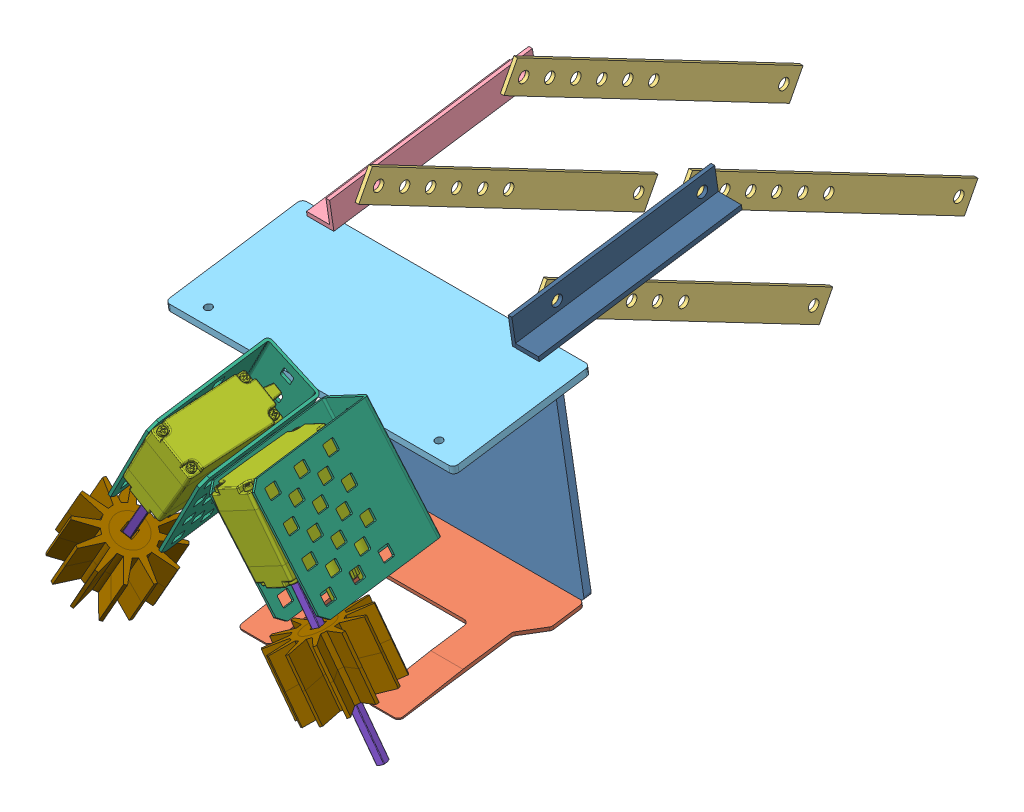
SolidWorks assembly Pyramid Intake, configuration Default. Lengths in mm.
Overall size (150.3 140.72 320.47).
19 component instances, 10 part files, 29 mates.
Components (placement in the parent):
- back-1: back [Default] at (51.2746 60.4405 44.4758) x (1 0 0) z (0 -0.146963 0.989142) size (85.5 99.5 3.17)
- BottomForklift-1: BottomForklift [Default] at (51.2746 -40.016 32.7601) x (1 0 0) z (0 -0.146963 0.989142) size (85.5 1.59 73.7)
- Circles 5.5in Inch Shaft Bar-1: Circles 5.5in Inch Shaft Bar [Default] at (81.5651 21.6246 -45.8337) x (0 0.885997 -0.463691) z (0 -0.463691 -0.885997) size (12.7 1.59 139.7)
- Circles 5.5in Inch Shaft Bar-2: Circles 5.5in Inch Shaft Bar [Default] at (81.5651 30.9788 -108.7925) x (0 0.885997 -0.463691) z (0 -0.463691 -0.885997) size (12.7 1.59 139.7)
- Circles 5.5in Inch Shaft Bar-3: Circles 5.5in Inch Shaft Bar [Default] at (1.9185 22.2168 -49.6344) x (0 0.885997 -0.463691) z (0 -0.463691 -0.885997) size (12.7 1.59 139.7)
- Circles 5.5in Inch Shaft Bar-4: Circles 5.5in Inch Shaft Bar [Default] at (1.9185 31.571 -112.5933) x (0 0.885997 -0.463691) z (0 -0.463691 -0.885997) size (12.7 1.59 139.7)
- Circles 3.5 inch Linkage-4: Circles 3.5 inch Linkage [Default] at (1.9185 61.0879 62.0444) x (0 0.989142 0.146963) z (0 -0.146963 0.989142) size (12.75 11.59 88.91)
- top-2: top [Default] at (45.9604 60.4405 44.4758) x (1 0 0) z (0 -0.146963 0.989142) size (125 3.17 60)
- VL-RACK-BRK RevA-1: VL-RACK-BRK RevA [Default] at (75.6784 37.9578 101.794) x (-0.866025 -0.494571 -0.073482) z (-0.5 0.856622 0.127274) size (24.56 52.4 50.8)
- VL-RACK-BRK RevA-2: VL-RACK-BRK RevA [Default] at (27.9082 38.1401 101.8211) x (-0.866025 0.494571 0.073482) z (0.5 0.856622 0.127274) size (24.56 52.4 50.8)
- VEX-2WIRE-MOTOR-1: VEX-2WIRE-MOTOR [Default] at (37.2345 49.19 137.8585) x (-0.036906 -0.095703 0.994726) z (0.523598 0.845979 0.100819) size (46.4 20 51.81)
- VEX-2WIRE-MOTOR-2: VEX-2WIRE-MOTOR [Default] at (66.0042 45.7522 136.293) x (0.02622 -0.1019 0.994449) z (-0.478039 0.872396 0.101997) size (46.4 20 51.81)
- SHAFT-4000-1: SHAFT-4000 [Default] at (87.1245 6.543 142.8927) x (0.260216 0.029754 0.965092) z (-0.478039 0.872396 0.101997) size (4.18 4.18 101.81)
- SHAFT-4000-2: SHAFT-4000 [Default] at (13.8193 10.8964 144.5121) x (0.829997 -0.479812 -0.284404) z (0.523598 0.845979 0.100819) size (4.18 4.18 101.81)
- INTAKE-ROLLER-1: INTAKE-ROLLER [Default] at (-2.7854 -15.9478 141.2978) x (0.248526 -0.038475 -0.967861) z (0.523598 0.845979 0.100819) size (38.1 38.1 12.7)
- INTAKE-ROLLER-2: INTAKE-ROLLER [Default] at (3.8643 -5.2039 142.5782) x (-0.192226 0.232592 -0.953389) z (0.523598 0.845979 0.100819) size (38.1 38.1 12.7)
- INTAKE-ROLLER-3: INTAKE-ROLLER [Default] at (91.181 -0.8787 142.0407) x (0.260216 0.029754 0.965092) z (0.478039 -0.872396 -0.101997) size (38.1 38.1 12.7)
- INTAKE-ROLLER-4: INTAKE-ROLLER [Default] at (97.2521 -11.9581 140.7453) x (-0.596407 -0.407651 0.691462) z (0.478039 -0.872396 -0.101997) size (38.1 38.1 12.7)
- Circles 3.5 inch Linkage-o-1: Circles 3.5 inch Linkage-o [Default] at (84.7401 60.4957 65.8452) x (0 0.989142 0.146963) z (0 -0.146963 0.989142) size (12.72 11.59 88.94)
Mates (geometry in assembly coordinates):
- Coincident5: coincident anti-aligned: plane of back-1 through (10.5246 -38.4457 32.9935) normal (0 -0.989142 -0.146963); plane of BottomForklift-1 through (32.2746 -42.9575 63.3601) normal (0 0.989142 0.146963)
- Coincident6: coincident aligned: plane of back-1 through (94.0246 57.9956 47.3224) normal (1 0 0); plane of BottomForklift-1 through (94.0246 -38.7396 34.9717) normal (1 0 0)
- Coincident41: coincident anti-aligned: plane of back-1 through (92.0246 -36.4674 33.2874) normal (0 -0.146963 0.989142); plane of BottomForklift-1 through (10.5246 -38.4457 32.9935) normal (0 0.146963 -0.989142)
- Concentric24: concentric anti-aligned: cylinder of Circles 5.5in Inch Shaft Bar-4 through (3.506 81.3019 -31.1847) axis (-1 0 0) radius 2.31; cylinder of Circles 3.5 inch Linkage-4 through (0.331 81.3019 -31.1847) axis (1 0 0) radius 2.31
- Concentric25: concentric anti-aligned: cylinder of Circles 5.5in Inch Shaft Bar-3 through (3.506 71.9477 31.7742) axis (-1 0 0) radius 2.31; cylinder of Circles 3.5 inch Linkage-4 through (0.331 71.9477 31.7742) axis (1 0 0) radius 2.31
- Coincident42: coincident anti-aligned: plane of Circles 5.5in Inch Shaft Bar-3 through (1.9185 22.2168 -49.6344) normal (-1 0 0); plane of Circles 3.5 inch Linkage-4 through (1.9185 61.0879 62.0444) normal (1 0 0)
- Coincident43: coincident anti-aligned: plane of Circles 5.5in Inch Shaft Bar-4 through (1.9185 31.571 -112.5933) normal (-1 0 0); plane of Circles 3.5 inch Linkage-4 through (1.9185 61.0879 62.0444) normal (1 0 0)
- Coincident63: coincident anti-aligned: plane of back-1 through (10.5246 59.9739 47.6163) normal (0 0.989142 0.146963); plane of top-2 through (-14.5396 51.9167 101.846) normal (0 -0.989142 -0.146963)
- Coincident64: coincident aligned: plane of back-1 through (92.0246 -36.0008 30.1469) normal (0 0.146963 -0.989142); plane of top-2 through (-14.5396 63.5811 44.9424) normal (0 0.146963 -0.989142)
- Coincident65: coincident anti-aligned: plane of top-2 through (-14.5396 54.7633 104.2909) normal (0 -0.146963 0.989142); plane of VL-RACK-BRK RevA-2 through (50.2319 54.4024 104.2373) normal (0 0.146963 -0.989142)
- Coincident67: coincident anti-aligned: plane of top-2 through (-14.5396 54.7633 104.2909) normal (0 -0.146963 0.989142); plane of VL-RACK-BRK RevA-1 through (72.6021 65.2119 105.8433) normal (0 0.146963 -0.989142)
- Angle2: planar angle = 1.047198 rad aligned: line of top-2 through (-14.5396 54.7633 104.2909) axis (1 0 0); line of VL-RACK-BRK RevA-1 through (73.614 65.4986 107.8889) axis (0.5 -0.856622 -0.127274)
- Angle3: planar angle = 1.047198 rad aligned: line of VL-RACK-BRK RevA-2 through (4.5726 22.1645 101.4504) axis (0.5 0.856622 0.127274); line of top-2 through (-14.5396 54.7633 104.2909) axis (1 0 0)
- Coincident74: coincident anti-aligned: line of VL-RACK-BRK RevA-2 through (29.397 54.9736 157.2976) axis (-0.5 -0.856622 -0.127274); line of VEX-2WIRE-MOTOR-1 through (18.0148 35.473 154.4002) axis (0.5 0.856622 0.127274)
- Coincident77: coincident anti-aligned: line of VL-RACK-BRK RevA-1 through (54.9422 43.7994 155.6373) axis (0.5 -0.856622 -0.127274); line of VEX-2WIRE-MOTOR-2 through (67.7297 21.8913 152.3823) axis (-0.5 0.856622 0.127274)
- Coincident99: coincident anti-aligned: plane of SHAFT-4000-1 through (61.0953 50.039 146.925) normal (-0.260216 -0.029754 -0.965092); plane of INTAKE-ROLLER-3 through (91.5496 -5.5891 140.4286) normal (0.260216 0.029754 0.965092)
- Coincident100: coincident anti-aligned: plane of SHAFT-4000-1 through (63.7588 51.588 146.1591) normal (0.838907 0.487893 -0.241235); plane of INTAKE-ROLLER-3 through (94.2341 -4.0278 139.6567) normal (-0.838907 -0.487893 0.241235)
- Coincident102: coincident anti-aligned: plane of INTAKE-ROLLER-3 through (94.2165 -6.4184 141.393) normal (0.478039 -0.872396 -0.101997); plane of INTAKE-ROLLER-4 through (94.2165 -6.4184 141.393) normal (-0.478039 0.872396 0.101997)
- Coincident103: coincident aligned: line of INTAKE-ROLLER-3 through (110.4029 1.771 147.2101) axis (-0.869601 -0.453744 -0.194707); line of INTAKE-ROLLER-4 through (110.4029 1.771 147.2101) axis (-0.869601 -0.453744 -0.194707)
- Coincident104: coincident aligned: line of INTAKE-ROLLER-3 through (97.8605 -5.4442 150.1393) axis (0.190922 -0.010142 0.981553); line of INTAKE-ROLLER-4 through (97.8605 -5.4442 150.1393) axis (0.190922 -0.010142 0.981553)
- Coincident105: coincident aligned: circle of Circles 5.5in Inch Shaft Bar-1; cylinder of Circles 3.5 inch Linkage-o-1 through (83.1526 71.3554 35.575) axis (1 0 0) radius 2.31
- Concentric26: concentric anti-aligned: cylinder of Circles 5.5in Inch Shaft Bar-2 through (83.1526 80.7096 -27.3839) axis (-1 0 0) radius 2.31; cylinder of Circles 3.5 inch Linkage-o-1 through (83.1526 80.7096 -27.3839) axis (1 0 0) radius 2.31
- Coincident108: coincident anti-aligned: plane of top-2 through (-14.5396 55.0572 102.3126) normal (0 0.989142 0.146963); plane of Circles 3.5 inch Linkage-o-1 through (94.7401 62.3279 53.377) normal (0 -0.989142 -0.146963)
- Coincident109: coincident anti-aligned: plane of Circles 3.5 inch Linkage-4 through (-9.669 75.9649 -38.4076) normal (0 -0.989142 -0.146963); plane of top-2 through (-14.5396 55.0572 102.3126) normal (0 0.989142 0.146963)
- Parallel8: parallel anti-aligned: line of Circles 5.5in Inch Shaft Bar-1 through (83.1526 15.1483 -85.5172) axis (0 0.463691 0.885997); line of Circles 5.5in Inch Shaft Bar-2 through (83.1526 78.028 -18.8134) axis (0 -0.463691 -0.885997)
- Coincident111: coincident anti-aligned: circle of Circles 5.5in Inch Shaft Bar-2; circle of Circles 3.5 inch Linkage-o-1
- Coincident112: coincident anti-aligned: circle of Circles 5.5in Inch Shaft Bar-1; circle of Circles 3.5 inch Linkage-o-1
- Parallel9: parallel aligned: line of Circles 5.5in Inch Shaft Bar-2 through (81.5651 24.5025 -148.476) axis (0 0.463691 0.885997); line of Circles 5.5in Inch Shaft Bar-4 through (3.506 25.0947 -152.2768) axis (0 0.463691 0.885997)
- Parallel10: parallel anti-aligned: line of Circles 5.5in Inch Shaft Bar-3 through (3.506 15.7405 -89.3179) axis (0 0.463691 0.885997); line of Circles 5.5in Inch Shaft Bar-4 through (3.506 78.6202 -22.6142) axis (0 -0.463691 -0.885997)
